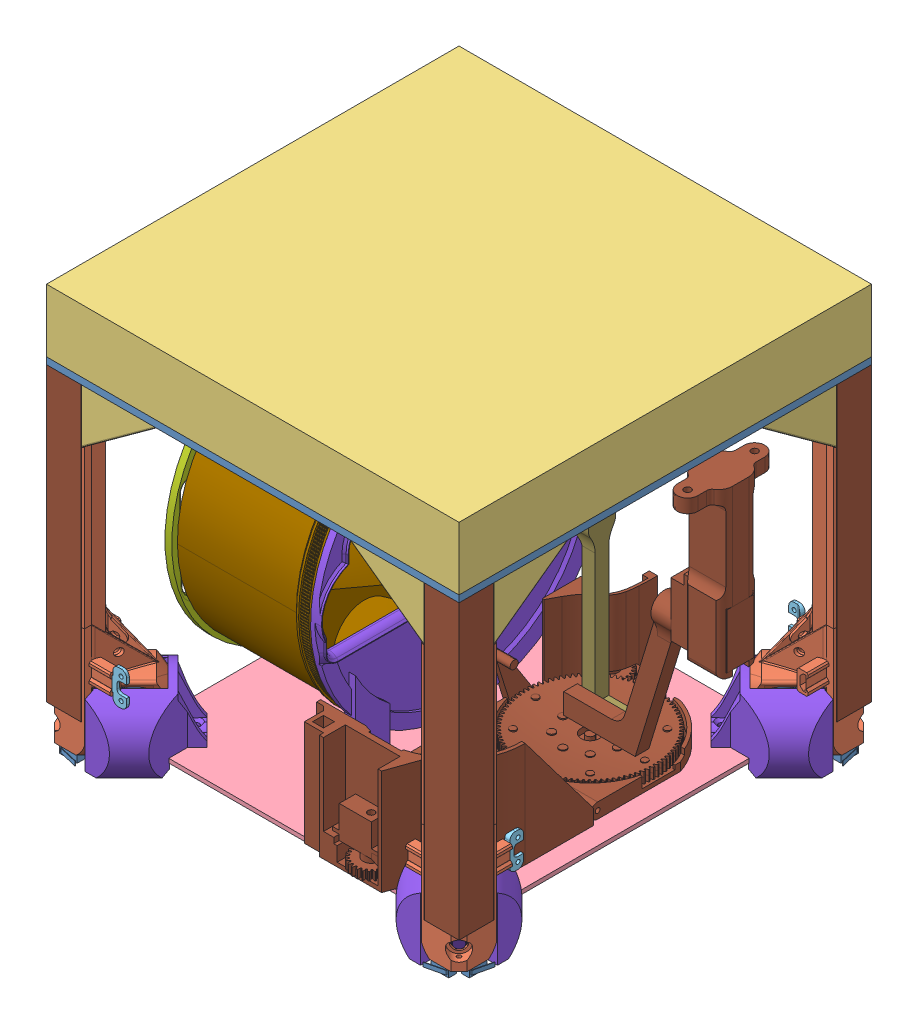
SolidWorks assembly MK7 IEEE BOT, configuration Default. Lengths in mm.
Overall size (425.24 302.29 425.24).
120 component instances, 33 part files, 52 mates.
Components (placement in the parent):
- MK5 Top Plate-1: MK5 Top Plate [Default] at (0 249 0) size (301.62 5 301.62)
- LEG assem MK5-1: LEG assem MK5 [Default] at (121.6905 25.4 121.6905) x (-0.707107 0 0.707107) z (-0.707107 0 -0.707107) size (113.86 301.29 113.86)
  - Omniwheel Mount-MK5-1: Omniwheel Mount-MK5 [Default] x (0 0 -1) z (1 0 0) size (67.69 82.93 55.08)
  - Leg Bracket MK5-1: Leg Bracket MK5 [Default] at (0 223.6 -41.1848) x (-0.707107 0 0.707107) z (-0.707107 0 -0.707107) size (80.51 40 80.51)
  - Omniwheel Hub-1: Omniwheel Hub [Default] at (0 0 13.95) x (-0.608761 -0.793353 0) z (0.793353 -0.608761 0) size (15.82 24.5 15.7)
  - TOF sensor mount-1: TOF sensor mount [Default] at (-9.5304 0 9.5304) x (0.707107 0 0.707107) z (-0.707107 0 0.707107) size (3.8 25 24.25)
  - Pinion Drive-1: Pinion Drive [Default] at (-0.7071 228.6 -26.6539) size (107.48 45 51.62)
  - helical gear_3_am-1: helical gear_3_am [Metric - LH Helical gear 1M 30T 25HA 20PA 4FW ---30N75H50L5.0N] at (0 249.6 4.5141) x (0 0 -1) z (0.567653 -0.823268 0) size (4 35.14 35.14)
  - Bottom Plate Bracket-1: Bottom Plate Bracket [Default] at (0 0 21.75) size (66.29 52.5 63.07)
  - Bearing Slider-1: Bearing Slider [Default] at (-0.7071 261.6 -26.6539) x (1 0 0) z (0 1 0) size (23.6 12.46 20)
  - 2in 14mm omniwheel-MK5-1: 2in 14mm omniwheel-MK5 [Default] at origin size (55.39 55.39 27.5)
  - Steel 90 degree MK5-1: Steel 90 degree MK5 [8982K151] at (0 120.65 -23.2243) x (-0.707107 0 -0.707107) z (0 1 0) size (25.4 25.4 213.6)
  - Nema17.step-2: Nema17.step [Default] at (22.8737 252.6 18.2122) x (0 -1 0) z (-1 0 0) size (42 57.7 46)
  - hex flange nut_am-2: hex flange nut_am [B18.2.2.4M - Hex flange nut, M6 x 1 --N] at (0 0 27.75) x (0.990831 -0.135106 0) z (0 0 1) size (14.2 14.2 6)
  - instrument ball bearing_68_am-4: instrument ball bearing_68_am [AFBMA 12.1.4.1 - 0070-14 - 12,SI,NC,12_68] at (0 0 -22.7198) x (0 0 1) z (-0.999767 0.021607 0) size (3.5 14 14)
  - 6mm G2T Pully Gear-1: 6mm G2T Pully Gear [Default] at (0 0 -9.25) x (0.996082 -0.088439 0) z (0.088439 0.996082 0) size (16 16 16)
  - 6mm G2T Pully Gear-2: 6mm G2T Pully Gear [Default] at (0 249.6 -30.45) x (-0.989152 0.146897 0) z (0.146897 0.989152 0) size (16 16 16)
  - Belt-1: Belt [Default] at (0 249.6 -23.35) x (-0.989152 0.146897 0) z (0 0 1) size (51.67 261.89 6)
  - instrument ball bearing_68_am-5: instrument ball bearing_68_am [AFBMA 12.1.4.1 - 0070-14 - 12,SI,NC,12_68] at (0 0 20) x (0 0 1) z (-0.999898 0.014309 0) size (3.5 14 14)
  - hex flange screw_am-1: hex flange screw_am [B18.2.3.4M - Hex flange screw, M5 x 0.8 x 35 --16N] at (0 0 -30.0698) x (0 0 1) z (-0.776229 0.630451 0) size (40.6 11.4 11.4)
  - hex flange screw_am-2: hex flange screw_am [B18.2.3.4M - Hex flange screw, M5 x 0.8 x 35 --16N] at (0 249.6 10.15) x (0 0 -1) z (-0.786653 -0.617395 0) size (40.6 11.4 11.4)
  - instrument ball bearing_68_am-6: instrument ball bearing_68_am [AFBMA 12.1.4.1 - 0070-14 - 12,SI,NC,12_68] at (0 251.6 -10.2) x (0 0 1) z (-0.998037 -0.06263 0) size (3.5 14 14)
  - instrument ball bearing_68_am-7: instrument ball bearing_68_am [AFBMA 12.1.4.1 - 0070-14 - 12,SI,NC,12_68] at (0 251.6 -2.2359) x (0 0 1) z (-0.682316 -0.731058 0) size (3.5 14 14)
  - hex screw_am-1: hex screw_am [B18.6.7M - M4 x 0.7 x 40 Indented HHMS --40N] at (5 274.6 -7.2179) x (0 -1 0) z (0 0 1) size (43 8.08 7)
  - Microswitch-1: Microswitch [Default] at (5.7276 -18.7296 -25.8406) x (0.707107 0 0.707107) z (-0.707107 0 0.707107) size (15.16 5.8 14.13)
  - Microswitch-2: Microswitch [Default] at (-5.7276 -12.9296 -25.8406) x (-0.707107 0 0.707107) z (0.707107 0 0.707107) size (15.16 5.8 14.13)
  - BeltShroud-1: BeltShroud [Default] at (0 70 0) x (0 0 -1) z (0 1 0) size (24.44 39.03 180.07)
- LEG assem MK5-2: LEG assem MK5 [Default] at (121.6905 25.4 -121.6905) x (0.707107 0 0.707107) z (-0.707107 0 0.707107) size (113.86 301.29 113.86)
  - Omniwheel Mount-MK5-1: Omniwheel Mount-MK5 [Default] x (0 0 -1) z (1 0 0) size (67.69 82.93 55.08)
  - Leg Bracket MK5-1: Leg Bracket MK5 [Default] at (0 223.6 -41.1848) x (-0.707107 0 0.707107) z (-0.707107 0 -0.707107) size (80.51 40 80.51)
  - Omniwheel Hub-1: Omniwheel Hub [Default] at (0 0 13.95) x (-0.608761 -0.793353 0) z (0.793353 -0.608761 0) size (15.82 24.5 15.7)
  - TOF sensor mount-1: TOF sensor mount [Default] at (-9.5304 0 9.5304) x (0.707107 0 0.707107) z (-0.707107 0 0.707107) size (3.8 25 24.25)
  - Pinion Drive-1: Pinion Drive [Default] at (-0.7071 228.6 -26.6539) size (107.48 45 51.62)
  - helical gear_3_am-1: helical gear_3_am [Metric - LH Helical gear 1M 30T 25HA 20PA 4FW ---30N75H50L5.0N] at (0 249.6 4.5141) x (0 0 -1) z (0.567653 -0.823268 0) size (4 35.14 35.14)
  - Bottom Plate Bracket-1: Bottom Plate Bracket [Default] at (0 0 21.75) size (66.29 52.5 63.07)
  - Bearing Slider-1: Bearing Slider [Default] at (-0.7071 261.6 -26.6539) x (1 0 0) z (0 1 0) size (23.6 12.46 20)
  - 2in 14mm omniwheel-MK5-1: 2in 14mm omniwheel-MK5 [Default] at origin size (55.39 55.39 27.5)
  - Steel 90 degree MK5-1: Steel 90 degree MK5 [8982K151] at (0 120.65 -23.2243) x (-0.707107 0 -0.707107) z (0 1 0) size (25.4 25.4 213.6)
  - Nema17.step-2: Nema17.step [Default] at (22.8737 252.6 18.2122) x (0 -1 0) z (-1 0 0) size (42 57.7 46)
  - hex flange nut_am-2: hex flange nut_am [B18.2.2.4M - Hex flange nut, M6 x 1 --N] at (0 0 27.75) x (0.990831 -0.135106 0) z (0 0 1) size (14.2 14.2 6)
  - instrument ball bearing_68_am-4: instrument ball bearing_68_am [AFBMA 12.1.4.1 - 0070-14 - 12,SI,NC,12_68] at (0 0 -22.7198) x (0 0 1) z (-0.999767 0.021607 0) size (3.5 14 14)
  - 6mm G2T Pully Gear-1: 6mm G2T Pully Gear [Default] at (0 0 -9.25) x (0.996082 -0.088439 0) z (0.088439 0.996082 0) size (16 16 16)
  - 6mm G2T Pully Gear-2: 6mm G2T Pully Gear [Default] at (0 249.6 -30.45) x (-0.989152 0.146897 0) z (0.146897 0.989152 0) size (16 16 16)
  - Belt-1: Belt [Default] at (0 249.6 -23.35) x (-0.989152 0.146897 0) z (0 0 1) size (51.67 261.89 6)
  - instrument ball bearing_68_am-5: instrument ball bearing_68_am [AFBMA 12.1.4.1 - 0070-14 - 12,SI,NC,12_68] at (0 0 20) x (0 0 1) z (-0.999898 0.014309 0) size (3.5 14 14)
  - hex flange screw_am-1: hex flange screw_am [B18.2.3.4M - Hex flange screw, M5 x 0.8 x 35 --16N] at (0 0 -30.0698) x (0 0 1) z (-0.776229 0.630451 0) size (40.6 11.4 11.4)
  - hex flange screw_am-2: hex flange screw_am [B18.2.3.4M - Hex flange screw, M5 x 0.8 x 35 --16N] at (0 249.6 10.15) x (0 0 -1) z (-0.786653 -0.617395 0) size (40.6 11.4 11.4)
  - instrument ball bearing_68_am-6: instrument ball bearing_68_am [AFBMA 12.1.4.1 - 0070-14 - 12,SI,NC,12_68] at (0 251.6 -10.2) x (0 0 1) z (-0.998037 -0.06263 0) size (3.5 14 14)
  - instrument ball bearing_68_am-7: instrument ball bearing_68_am [AFBMA 12.1.4.1 - 0070-14 - 12,SI,NC,12_68] at (0 251.6 -2.2359) x (0 0 1) z (-0.682316 -0.731058 0) size (3.5 14 14)
  - hex screw_am-1: hex screw_am [B18.6.7M - M4 x 0.7 x 40 Indented HHMS --40N] at (5 274.6 -7.2179) x (0 -1 0) z (0 0 1) size (43 8.08 7)
  - Microswitch-1: Microswitch [Default] at (5.7276 -18.7296 -25.8406) x (0.707107 0 0.707107) z (-0.707107 0 0.707107) size (15.16 5.8 14.13)
  - Microswitch-2: Microswitch [Default] at (-5.7276 -12.9296 -25.8406) x (-0.707107 0 0.707107) z (0.707107 0 0.707107) size (15.16 5.8 14.13)
  - BeltShroud-1: BeltShroud [Default] at (0 70 0) x (0 0 -1) z (0 1 0) size (24.44 39.03 180.07)
- LEG assem MK5-3: LEG assem MK5 [Default] at (-121.6905 25.4 -121.6905) x (0.707107 0 -0.707107) z (0.707107 0 0.707107) size (113.86 301.29 113.86)
  - Omniwheel Mount-MK5-1: Omniwheel Mount-MK5 [Default] x (0 0 -1) z (1 0 0) size (67.69 82.93 55.08)
  - Leg Bracket MK5-1: Leg Bracket MK5 [Default] at (0 223.6 -41.1848) x (-0.707107 0 0.707107) z (-0.707107 0 -0.707107) size (80.51 40 80.51)
  - Omniwheel Hub-1: Omniwheel Hub [Default] at (0 0 13.95) x (-0.608761 -0.793353 0) z (0.793353 -0.608761 0) size (15.82 24.5 15.7)
  - TOF sensor mount-1: TOF sensor mount [Default] at (-9.5304 0 9.5304) x (0.707107 0 0.707107) z (-0.707107 0 0.707107) size (3.8 25 24.25)
  - Pinion Drive-1: Pinion Drive [Default] at (-0.7071 228.6 -26.6539) size (107.48 45 51.62)
  - helical gear_3_am-1: helical gear_3_am [Metric - LH Helical gear 1M 30T 25HA 20PA 4FW ---30N75H50L5.0N] at (0 249.6 4.5141) x (0 0 -1) z (0.567653 -0.823268 0) size (4 35.14 35.14)
  - Bottom Plate Bracket-1: Bottom Plate Bracket [Default] at (0 0 21.75) size (66.29 52.5 63.07)
  - Bearing Slider-1: Bearing Slider [Default] at (-0.7071 261.6 -26.6539) x (1 0 0) z (0 1 0) size (23.6 12.46 20)
  - 2in 14mm omniwheel-MK5-1: 2in 14mm omniwheel-MK5 [Default] at origin size (55.39 55.39 27.5)
  - Steel 90 degree MK5-1: Steel 90 degree MK5 [8982K151] at (0 120.65 -23.2243) x (-0.707107 0 -0.707107) z (0 1 0) size (25.4 25.4 213.6)
  - Nema17.step-2: Nema17.step [Default] at (22.8737 252.6 18.2122) x (0 -1 0) z (-1 0 0) size (42 57.7 46)
  - hex flange nut_am-2: hex flange nut_am [B18.2.2.4M - Hex flange nut, M6 x 1 --N] at (0 0 27.75) x (0.990831 -0.135106 0) z (0 0 1) size (14.2 14.2 6)
  - instrument ball bearing_68_am-4: instrument ball bearing_68_am [AFBMA 12.1.4.1 - 0070-14 - 12,SI,NC,12_68] at (0 0 -22.7198) x (0 0 1) z (-0.999767 0.021607 0) size (3.5 14 14)
  - 6mm G2T Pully Gear-1: 6mm G2T Pully Gear [Default] at (0 0 -9.25) x (0.996082 -0.088439 0) z (0.088439 0.996082 0) size (16 16 16)
  - 6mm G2T Pully Gear-2: 6mm G2T Pully Gear [Default] at (0 249.6 -30.45) x (-0.989152 0.146897 0) z (0.146897 0.989152 0) size (16 16 16)
  - Belt-1: Belt [Default] at (0 249.6 -23.35) x (-0.989152 0.146897 0) z (0 0 1) size (51.67 261.89 6)
  - instrument ball bearing_68_am-5: instrument ball bearing_68_am [AFBMA 12.1.4.1 - 0070-14 - 12,SI,NC,12_68] at (0 0 20) x (0 0 1) z (-0.999898 0.014309 0) size (3.5 14 14)
  - hex flange screw_am-1: hex flange screw_am [B18.2.3.4M - Hex flange screw, M5 x 0.8 x 35 --16N] at (0 0 -30.0698) x (0 0 1) z (-0.776229 0.630451 0) size (40.6 11.4 11.4)
  - hex flange screw_am-2: hex flange screw_am [B18.2.3.4M - Hex flange screw, M5 x 0.8 x 35 --16N] at (0 249.6 10.15) x (0 0 -1) z (-0.786653 -0.617395 0) size (40.6 11.4 11.4)
  - instrument ball bearing_68_am-6: instrument ball bearing_68_am [AFBMA 12.1.4.1 - 0070-14 - 12,SI,NC,12_68] at (0 251.6 -10.2) x (0 0 1) z (-0.998037 -0.06263 0) size (3.5 14 14)
  - instrument ball bearing_68_am-7: instrument ball bearing_68_am [AFBMA 12.1.4.1 - 0070-14 - 12,SI,NC,12_68] at (0 251.6 -2.2359) x (0 0 1) z (-0.682316 -0.731058 0) size (3.5 14 14)
  - hex screw_am-1: hex screw_am [B18.6.7M - M4 x 0.7 x 40 Indented HHMS --40N] at (5 274.6 -7.2179) x (0 -1 0) z (0 0 1) size (43 8.08 7)
  - Microswitch-1: Microswitch [Default] at (5.7276 -18.7296 -25.8406) x (0.707107 0 0.707107) z (-0.707107 0 0.707107) size (15.16 5.8 14.13)
  - Microswitch-2: Microswitch [Default] at (-5.7276 -12.9296 -25.8406) x (-0.707107 0 0.707107) z (0.707107 0 0.707107) size (15.16 5.8 14.13)
  - BeltShroud-1: BeltShroud [Default] at (0 70 0) x (0 0 -1) z (0 1 0) size (24.44 39.03 180.07)
- LEG assem MK5-4: LEG assem MK5 [Default] at (-121.6905 25.4 121.6905) x (-0.707107 0 -0.707107) z (0.707107 0 -0.707107) size (113.86 301.29 113.86)
  - Omniwheel Mount-MK5-1: Omniwheel Mount-MK5 [Default] x (0 0 -1) z (1 0 0) size (67.69 82.93 55.08)
  - Leg Bracket MK5-1: Leg Bracket MK5 [Default] at (0 223.6 -41.1848) x (-0.707107 0 0.707107) z (-0.707107 0 -0.707107) size (80.51 40 80.51)
  - Omniwheel Hub-1: Omniwheel Hub [Default] at (0 0 13.95) x (-0.608761 -0.793353 0) z (0.793353 -0.608761 0) size (15.82 24.5 15.7)
  - TOF sensor mount-1: TOF sensor mount [Default] at (-9.5304 0 9.5304) x (0.707107 0 0.707107) z (-0.707107 0 0.707107) size (3.8 25 24.25)
  - Pinion Drive-1: Pinion Drive [Default] at (-0.7071 228.6 -26.6539) size (107.48 45 51.62)
  - helical gear_3_am-1: helical gear_3_am [Metric - LH Helical gear 1M 30T 25HA 20PA 4FW ---30N75H50L5.0N] at (0 249.6 4.5141) x (0 0 -1) z (0.567653 -0.823268 0) size (4 35.14 35.14)
  - Bottom Plate Bracket-1: Bottom Plate Bracket [Default] at (0 0 21.75) size (66.29 52.5 63.07)
  - Bearing Slider-1: Bearing Slider [Default] at (-0.7071 261.6 -26.6539) x (1 0 0) z (0 1 0) size (23.6 12.46 20)
  - 2in 14mm omniwheel-MK5-1: 2in 14mm omniwheel-MK5 [Default] at origin size (55.39 55.39 27.5)
  - Steel 90 degree MK5-1: Steel 90 degree MK5 [8982K151] at (0 120.65 -23.2243) x (-0.707107 0 -0.707107) z (0 1 0) size (25.4 25.4 213.6)
  - Nema17.step-2: Nema17.step [Default] at (22.8737 252.6 18.2122) x (0 -1 0) z (-1 0 0) size (42 57.7 46)
  - hex flange nut_am-2: hex flange nut_am [B18.2.2.4M - Hex flange nut, M6 x 1 --N] at (0 0 27.75) x (0.990831 -0.135106 0) z (0 0 1) size (14.2 14.2 6)
  - instrument ball bearing_68_am-4: instrument ball bearing_68_am [AFBMA 12.1.4.1 - 0070-14 - 12,SI,NC,12_68] at (0 0 -22.7198) x (0 0 1) z (-0.999767 0.021607 0) size (3.5 14 14)
  - 6mm G2T Pully Gear-1: 6mm G2T Pully Gear [Default] at (0 0 -9.25) x (0.996082 -0.088439 0) z (0.088439 0.996082 0) size (16 16 16)
  - 6mm G2T Pully Gear-2: 6mm G2T Pully Gear [Default] at (0 249.6 -30.45) x (-0.989152 0.146897 0) z (0.146897 0.989152 0) size (16 16 16)
  - Belt-1: Belt [Default] at (0 249.6 -23.35) x (-0.989152 0.146897 0) z (0 0 1) size (51.67 261.89 6)
  - instrument ball bearing_68_am-5: instrument ball bearing_68_am [AFBMA 12.1.4.1 - 0070-14 - 12,SI,NC,12_68] at (0 0 20) x (0 0 1) z (-0.999898 0.014309 0) size (3.5 14 14)
  - hex flange screw_am-1: hex flange screw_am [B18.2.3.4M - Hex flange screw, M5 x 0.8 x 35 --16N] at (0 0 -30.0698) x (0 0 1) z (-0.776229 0.630451 0) size (40.6 11.4 11.4)
  - hex flange screw_am-2: hex flange screw_am [B18.2.3.4M - Hex flange screw, M5 x 0.8 x 35 --16N] at (0 249.6 10.15) x (0 0 -1) z (-0.786653 -0.617395 0) size (40.6 11.4 11.4)
  - instrument ball bearing_68_am-6: instrument ball bearing_68_am [AFBMA 12.1.4.1 - 0070-14 - 12,SI,NC,12_68] at (0 251.6 -10.2) x (0 0 1) z (-0.998037 -0.06263 0) size (3.5 14 14)
  - instrument ball bearing_68_am-7: instrument ball bearing_68_am [AFBMA 12.1.4.1 - 0070-14 - 12,SI,NC,12_68] at (0 251.6 -2.2359) x (0 0 1) z (-0.682316 -0.731058 0) size (3.5 14 14)
  - hex screw_am-1: hex screw_am [B18.6.7M - M4 x 0.7 x 40 Indented HHMS --40N] at (5 274.6 -7.2179) x (0 -1 0) z (0 0 1) size (43 8.08 7)
  - Microswitch-1: Microswitch [Default] at (5.7276 -18.7296 -25.8406) x (0.707107 0 0.707107) z (-0.707107 0 0.707107) size (15.16 5.8 14.13)
  - Microswitch-2: Microswitch [Default] at (-5.7276 -12.9296 -25.8406) x (-0.707107 0 0.707107) z (0.707107 0 0.707107) size (15.16 5.8 14.13)
  - BeltShroud-1: BeltShroud [Default] at (0 70 0) x (0 0 -1) z (0 1 0) size (24.44 39.03 180.07)
- Leg Bracket MK5-1: Leg Bracket MK5 [Default] at (-150.8125 249 150.8125) size (80.51 40 80.51)
- Bottom Plate Bracket-1: Bottom Plate Bracket [Default] at (106.3109 25.4 -106.3109) x (0.707107 0 0.707107) z (-0.707107 0 0.707107) size (66.29 52.5 63.07)
- TopCover-1: TopCover [Default] at (0 254 0) x (1 0 0) z (0 1 0) size (301.63 301.63 46)
- Bottom Plate21-1: Bottom Plate21 [Default] at (-75.998 15.4 -153.7106) x (-0.707107 0 0.707107) z (0 -1 0) size (300.69 300.69 3)
- Nema14Pancake Stepper-1: Nema14Pancake Stepper [Default] at (-22.1225 272 0) x (0 0 -1) z (0 1 0) size (51 23.8 36)
- 3764N114_High-Strength Gt Timing Belt Pulley-1: 3764N114_High-Strength Gt Timing Belt Pulley [3764N114] at (-20.5438 272 0) x (0 -0.930392 -0.366566) z (-1 0 0) size (30.73 30.73 9.91)
- EleFlipAss.step-2: EleFlipAss.step [Default] at (36.9866 19.2914 -10.575) x (1 0 0) z (0 1 0) size (148 245.19 83.5) (hidden)
- DrumHolderBackPlate.step-1: DrumHolderBackPlate.step [Default] at (-105.0625 135.4 0) x (0 0 1) z (-1 0 0) size (210 233.1 15.65)
- 3Duck 3Cyl twist MK5-2: 3Duck 3Cyl twist MK5 [Non-Split] at (-105.0625 135.4 0) x (0 -0.264931 -0.964267) z (1 0 0) size (208.49 208.49 100.02) (hidden)
- twist_inside_plate-2: twist_inside_plate [Default] at (-3.5625 135.4 0) size (8.95 233.6 210)
- StorageDrum3-1: StorageDrum3 [Default] at (-104.0625 135.4 0) x (0 0.009925 -0.999951) z (1 0 0) size (208.49 208.49 100.03)
- Part2^MK7 IEEE BOT-1: Part2^MK7 IEEE BOT [Default] at origin (virtual)
- NylonBushing-1: NylonBushing [Default] at (-104.8625 135.4 0) x (0 0.017134 0.999853) z (-1 0 0) size (30 30 1)
- FrontCollect.step-1: FrontCollect.step [Default] at (21.2525 12.4 1.0438) x (1 0 0) z (0 1 0) size (167.04 245.19 235.1)
- DuckKicker-1: DuckKicker [Default] at (145.1674 31.2268 -89.4371) x (-1 0 0) z (0 1 0) size (73.71 64 222.88)
Mates (geometry in assembly coordinates):
- Coincident1: coincident aligned: plane of MK5 Top Plate-1 through (0 249 0) normal (0 0 1)
- Coincident2: coincident aligned: plane of MK5 Top Plate-1 through (0 249 0) normal (1 0 0)
- Distance1: distance = 254 mm aligned: plane of MK5 Top Plate-1 through (0 254 0) normal (0 1 0)
- Coincident3: coincident aligned: plane of MK5 Top Plate-1 through (-150.8125 254 150.8125) normal (0 0 1); plane of LEG assem MK5-1/Steel 90 degree MK5-1 through (125.4125 298.45 150.8125) normal (0 0 1)
- Coincident5: coincident aligned: plane of MK5 Top Plate-1 through (150.8125 254 150.8125) normal (1 0 0); plane of LEG assem MK5-1/Steel 90 degree MK5-1 through (150.8125 298.45 150.8125) normal (1 0 0)
- Coincident6: coincident aligned: plane of LEG assem MK5-1 through (121.6905 0 121.6905) normal (0 1 0)
- Coincident11: coincident aligned: plane of MK5 Top Plate-1 through (-150.8125 254 -150.8125) normal (0 0 -1); plane of LEG assem MK5-2/Steel 90 degree MK5-1 through (150.8125 298.45 -150.8125) normal (0 0 -1)
- Coincident12: coincident aligned: plane of MK5 Top Plate-1 through (150.8125 254 150.8125) normal (1 0 0); plane of LEG assem MK5-2/Steel 90 degree MK5-1 through (150.8125 298.45 -125.4125) normal (1 0 0)
- Coincident14: coincident aligned: plane of LEG assem MK5-2/Steel 90 degree MK5-1 through (150.8125 298.45 -150.8125) normal (0 0 -1); plane of LEG assem MK5-3/Steel 90 degree MK5-1 through (-125.4125 298.45 -150.8125) normal (0 0 -1)
- Coincident15: coincident aligned: plane of MK5 Top Plate-1 through (-150.8125 254 150.8125) normal (-1 0 0); plane of LEG assem MK5-3/Steel 90 degree MK5-1 through (-150.8125 298.45 -150.8125) normal (-1 0 0)
- Coincident17: coincident aligned: plane of MK5 Top Plate-1 through (-150.8125 254 150.8125) normal (-1 0 0); plane of LEG assem MK5-4/Steel 90 degree MK5-1 through (-150.8125 298.45 125.4125) normal (-1 0 0)
- Coincident18: coincident aligned: plane of MK5 Top Plate-1 through (-150.8125 254 150.8125) normal (0 0 1); plane of LEG assem MK5-4/Steel 90 degree MK5-1 through (-150.8125 298.45 150.8125) normal (0 0 1)
- Coincident29: coincident aligned: plane of MK5 Top Plate-1 through (-150.8125 254 150.8125) normal (0 0 1); plane of Leg Bracket MK5-1 through (-150.8125 249 150.8125) normal (0 0 1)
- Coincident30: coincident anti-aligned: plane of LEG assem MK5-4/Steel 90 degree MK5-1 through (-150.8125 298.45 125.4125) normal (-1 0 0); plane of Leg Bracket MK5-1 through (-150.8125 249 150.8125) normal (1 0 0)
- Coincident31: coincident anti-aligned: plane of MK5 Top Plate-1 through (0 249 0) normal (0 -1 0); plane of Leg Bracket MK5-1 through (-150.8125 249 150.8125) normal (0 1 0)
- Tangent1: tangent anti-aligned: plane of MK5 Top Plate-1 through (0 254 0) normal (0 1 0); cylinder of Nema14Pancake Stepper-1 through (-24.6225 272 0) axis (1 0 0) radius 18
- Coincident49: coincident: line of Nema14Pancake Stepper-1 through (-15.3225 272 0) axis (-1 0 0)
- Parallel2: parallel aligned: plane of MK5 Top Plate-1 through (0 254 0) normal (0 1 0); plane of Nema14Pancake Stepper-1 through (-22.1225 272 0) normal (0 1 0)
- Concentric3: concentric aligned: cylinder of Nema14Pancake Stepper-1 through (-15.3225 272 0) axis (-1 0 0) radius 2.5; cylinder of 3764N114_High-Strength Gt Timing Belt Pulley-1 through (-29.6751 272 0) axis (-1 0 0) radius 15.367
- Coincident50: coincident anti-aligned: plane of Nema14Pancake Stepper-1 through (-15.3225 272 0) normal (1 0 0); plane of 3764N114_High-Strength Gt Timing Belt Pulley-1 through (-15.3225 270.5905 2.3366) normal (-1 0 0)
- Coincident56: coincident anti-aligned: plane of MK5 Top Plate-1 through (0 249 0) normal (0 -1 0); plane of LEG assem MK5-3/Leg Bracket MK5-1 through (-150.8125 249 -150.8125) normal (0 1 0)
- Coincident57: coincident anti-aligned: plane of MK5 Top Plate-1 through (0 249 0) normal (0 -1 0); plane of LEG assem MK5-4/Leg Bracket MK5-1 through (-150.8125 249 150.8125) normal (0 1 0)
- Coincident58: coincident anti-aligned: plane of MK5 Top Plate-1 through (0 249 0) normal (0 -1 0); plane of LEG assem MK5-2/Leg Bracket MK5-1 through (150.8125 249 -150.8125) normal (0 1 0)
- InPlace5: in place: plane of LEG assem MK5-2/Omniwheel Mount-MK5-1 through (106.3109 25.4 -106.3109) normal (-0.707107 0 0.707107); plane of ? through (106.3109 0 -106.3109) normal (-0.707107 0 0.707107); moOrthogonalPlaneRef_w of LEG assem MK5-2/Omniwheel Mount-MK5-1 through (106.3109 25.4 -106.3109) normal (-0.707107 0 0.707107); plane of ? through (106.3109 0 -106.3109) normal (0 1 0); plane of LEG assem MK5-2/Omniwheel Mount-MK5-1 through (106.3109 25.4 -106.3109) normal (-0.707107 0 0.707107); plane of ? through (106.3109 0 -106.3109) normal (0.707107 0 0.707107); plane of LEG assem MK5-2/Omniwheel Mount-MK5-1 through (106.3109 25.4 -106.3109) normal (-0.707107 0 0.707107); unknown of ?
- Coincident59: coincident aligned: plane of LEG assem MK5-2/Omniwheel Mount-MK5-1; plane of Bottom Plate Bracket-1
- Coincident60: coincident aligned: moOrthogonalPlaneRef_w of LEG assem MK5-2/Omniwheel Mount-MK5-1 through (106.3109 25.4 -106.3109) normal (0 1 0); plane of Bottom Plate Bracket-1 through (106.3109 25.4 -106.3109) normal (0 1 0)
- Coincident61: coincident anti-aligned: moOrthogonalPlaneRef_w of LEG assem MK5-2/Omniwheel Mount-MK5-1 through (106.3109 25.4 -106.3109) normal (-0.707107 0 -0.707107); plane of Bottom Plate Bracket-1 through (106.3109 25.4 -106.3109) normal (0.707107 0 0.707107)
- Coincident59: coincident aligned: circle of LEG assem MK5-4/Bottom Plate Bracket-1; cylinder of Bottom Plate21-1 through (-92.6454 12.4 99.4703) axis (0 1 0) radius 2.25
- Coincident60: coincident anti-aligned: plane of LEG assem MK5-4/Bottom Plate Bracket-1 through (-100.1237 15.4 112.4981) normal (0 -1 0); plane of Bottom Plate21-1 through (-75.998 15.4 -153.7106) normal (0 1 0)
- Concentric6: concentric aligned: cylinder of LEG assem MK5-2/Bottom Plate Bracket-1 through (99.4703 9.4 -92.6454) axis (0 1 0) radius 2.25; cylinder of Bottom Plate21-1 through (99.4703 12.4 -92.6454) axis (0 1 0) radius 2.25
- InPlace6: in place: plane of MK5 Top Plate-1 through (0 254 0) normal (0 1 0); plane of TopCover-1 through (0 254 0) normal (0 1 0); plane of MK5 Top Plate-1 through (0 254 0) normal (0 1 0); plane of TopCover-1 through (0 254 0) normal (0 0 -1); plane of MK5 Top Plate-1 through (0 254 0) normal (0 1 0); plane of TopCover-1 through (0 254 0) normal (1 0 0); plane of MK5 Top Plate-1 through (0 254 0) normal (0 1 0); unknown of TopCover-1
- Coincident63: coincident aligned: plane of MK5 Top Plate-1; plane of ?
- Coincident64: coincident aligned: moOrthogonalPlaneRef_w of MK5 Top Plate-1 through (0 254 0) normal (0 0 -1); plane of TopCover-1 through (0 254 0) normal (0 0 -1)
- Coincident65: coincident anti-aligned: moOrthogonalPlaneRef_w of MK5 Top Plate-1 through (0 254 0) normal (-1 0 0); plane of TopCover-1 through (0 254 0) normal (1 0 0)
- Coincident62: coincident aligned: plane of DrumHolderBackPlate.step-1 through (-105.0625 135.4 0) normal (0 0 1)
- Coincident65: coincident anti-aligned: plane of DrumHolderBackPlate.step-1 through (-105.0625 135.4 0) normal (1 0 0); plane of 3Duck 3Cyl twist MK5-2 through (-105.0625 135.4 0) normal (-1 0 0)
- Concentric8: concentric aligned: circle of DrumHolderBackPlate.step-1; cylinder of 3Duck 3Cyl twist MK5-2 through (-5.0511 135.4 0) axis (-1 0 0) radius 5
- Concentric9: concentric aligned: cylinder of 3Duck 3Cyl twist MK5-2 through (-5.0511 135.4 0) axis (-1 0 0) radius 5; cylinder of twist_inside_plate-2 through (-0.5625 135.4 0) axis (-1 0 0) radius 4
- Distance3: distance = 40.75 mm aligned: plane of DrumHolderBackPlate.step-1 through (-110.0625 135.4 0) normal (-1 0 0); plane of LEG assem MK5-3/Steel 90 degree MK5-1 through (-150.8125 298.45 -150.8125) normal (-1 0 0)
- Parallel3: parallel aligned: plane of LEG assem MK5-4/Steel 90 degree MK5-1 through (-150.8125 298.45 150.8125) normal (0 0 1); plane of LEG assem MK5-1/Steel 90 degree MK5-1 through (125.4125 298.45 150.8125) normal (0 0 1)
- Coincident68: coincident anti-aligned: plane of MK5 Top Plate-1 through (0 249 0) normal (0 -1 0); plane of DrumHolderBackPlate.step-1 through (-132.3125 249 79.2101) normal (0 1 0)
- Concentric10: concentric aligned: cylinder of twist_inside_plate-2 through (-0.5625 135.4 0) axis (-1 0 0) radius 4; cylinder of StorageDrum3-1 through (-4.0511 135.4 0) axis (-1 0 0) radius 5
- Distance4: distance = 1 mm anti-aligned: plane of StorageDrum3-1 through (-104.0625 135.4 0) normal (-1 0 0); plane of DrumHolderBackPlate.step-1 through (-105.0625 135.4 0) normal (1 0 0)
- Concentric11: concentric anti-aligned: cylinder of DrumHolderBackPlate.step-1 through (-108.0625 135.4 0) axis (1 0 0) radius 4.2; circle of NylonBushing-1
- Distance5: distance = 0.2 mm aligned: plane of DrumHolderBackPlate.step-1 through (-105.0625 135.4 0) normal (1 0 0); plane of NylonBushing-1 through (-104.8625 135.4 0) normal (1 0 0)
- Distance7: distance = 0.5 mm anti-aligned: plane of twist_inside_plate-2 through (-3.5625 135.4 0) normal (-1 0 0); plane of StorageDrum3-1 through (-4.0625 135.4 0) normal (1 0 0)
- Parallel4: parallel aligned: plane of Bottom Plate21-1 through (-75.998 15.4 -153.7106) normal (0 1 0); plane of twist_inside_plate-2 through (-110.5183 113.4 25.38) normal (0 1 0)
- Coincident72: coincident anti-aligned: plane of Bottom Plate21-1 through (-75.998 15.4 -153.7106) normal (0 1 0); plane of FrontCollect.step-1 through (21.2525 15.4 1.0438) normal (0 -1 0)
- Distance8: distance = 0.5 mm anti-aligned: plane of twist_inside_plate-2 through (4.4375 249.001 80) normal (1 0 0); plane of FrontCollect.step-1 through (4.9375 18.4 59.0238) normal (-1 0 0)
- Coincident74: coincident anti-aligned: plane of twist_inside_plate-2 through (-0.5625 135.4 0) normal (1 0 0); plane of DuckKicker-1 through (-0.5625 161.5 -49.4898) normal (-1 0 0)
- Parallel5: parallel aligned: plane of twist_inside_plate-2 through (-3.5625 249 -79.2101) normal (0 0 -1); plane of DuckKicker-1 through (-0.5625 171.5 -59.4898) normal (0 0 -1)
- Distance9: distance = 67.5 mm anti-aligned: plane of DuckKicker-1 through (-0.5625 181.5 -49.4898) normal (0 1 0); plane of MK5 Top Plate-1 through (0 249 0) normal (0 -1 0)
